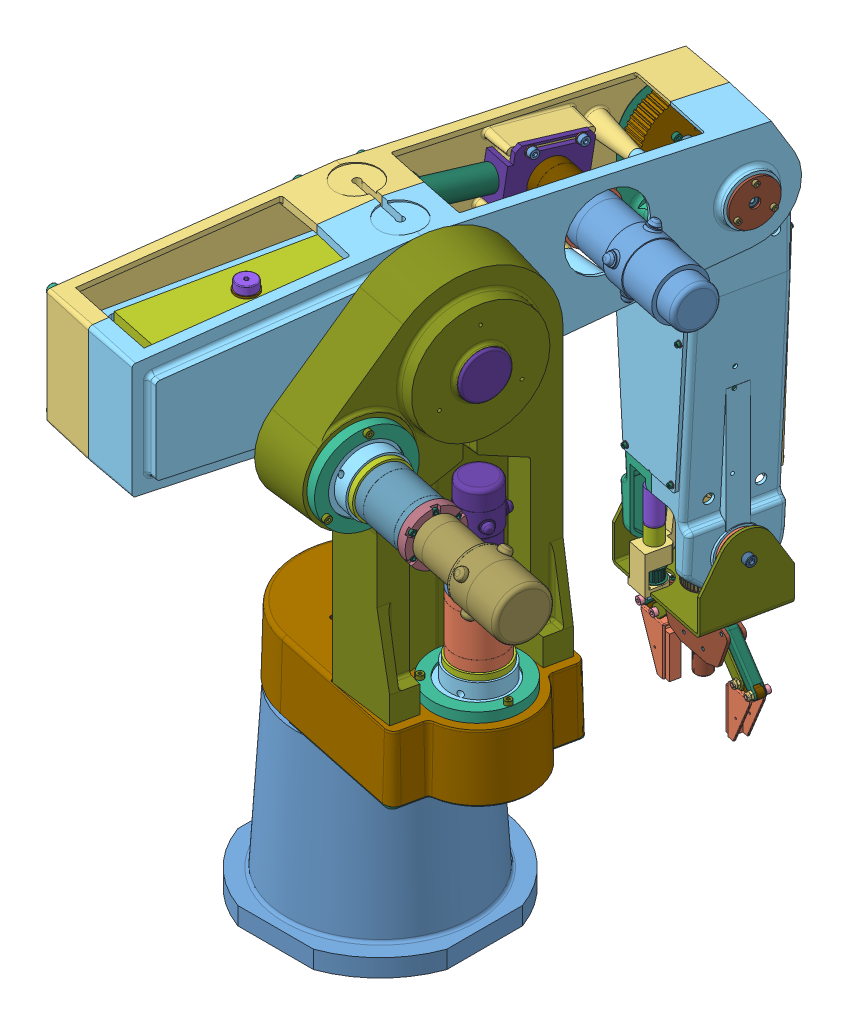
SolidWorks assembly Robot 2, configuration Défaut. Lengths in mm. (continued)
Components (placement in the parent): (continued)
- SE-AvtBras-1: SE-AvtBras [Défaut] at (55.1759 532.5 -274.5106) x (0 1 0) z (-0.978958 0 -0.204064) size (419.1 115.2 105.3)
  - AvtBrasD-1: AvtBrasD [Défaut] at origin size (406.26 90.38 52)
  - AvtBrasG-1: AvtBrasG [Défaut] at (-0.1665 0.8325 0) size (406.15 90.36 52)
  - parallel pin hardened_iso-1: parallel pin hardened_iso [Goupille  - 4 x 16 - A - St] at (-265.5 30.1675 -8) x (0 0 1) z (-0.010471 -0.999945 0) size (16 4 4)
  - Vis C HC, M 6x70-1: Vis C HC, M 6x70 [Défaut] at (-65 -16 45.5) x (1 0 0) z (0 -1 0) size (10 76 10)
  - GoupillePosition-1: GoupillePosition [Défaut] at (-65 -16 0.2) x (0 0 1) z (-0.991523 0.129934 0) size (10 8 8)
  - Support moteur-1: Support moteur [Défaut] at (-98.931 38.4675 -40.5) x (0 0 1) z (1 0 0) size (77 78 106) (hidden)
  - socket head cap screw_iso-1: socket head cap screw_iso [Vis CHC M5 x 12 --- 12N] at (-173.5 -4.3325 -27.8) x (0 0 -1) z (0.120643 0.992696 0) size (17 8.5 8.5)
  - socket head cap screw_iso-2: socket head cap screw_iso [Vis CHC M5 x 12 --- 12N] at (-153.5 -4.3325 -27.8) x (0 0 -1) z (0.975756 0.218862 0) size (17 8.5 8.5)
  - plain washer large grade ac_iso-1: plain washer large grade ac_iso [Rondelle M5 Washer ISO 7093 - 5] at (-173.5 -4.3325 -32.8) x (0 0 1) z (-1 0 0) size (1.2 15 15)
  - plain washer large grade ac_iso-3: plain washer large grade ac_iso [Rondelle M5 Washer ISO 7093 - 5] at (-153.5 -4.3325 -32.8) x (0 0 1) z (-1 0 0) size (1.2 15 15)
  - Poulie_M300-006-1: Poulie_M300-006 [Défaut] at (0 0 39) x (0 0 1) z (-0.707107 -0.707107 0) size (22 81.46 81.46)
  - Goupille Cylindrique type A  , 4x24-1: Goupille Cylindrique type A  , 4x24 [Défaut] at (9.1924 9.1924 26.3203) x (0.697271 -0.716808 0) z (0 0 1) size (4 4 24)
  - Goupille Cylindrique type A  , 4x24-3: Goupille Cylindrique type A  , 4x24 [Défaut] at (-9.1924 -9.1924 24.7225) x (-0.993131 -0.117006 0) z (0 0 1) size (4 4 24)
  - socket head cap screw_iso-3: socket head cap screw_iso [Vis CHC M4 x 25 ] at (-9.1924 9.1924 20) x (0 0 1) z (-1 0 0) size (29 7 7)
  - socket head cap screw_iso-4: socket head cap screw_iso [Vis CHC M4 x 25 ] at (9.1924 -9.1924 20) x (0 0 1) z (-1 0 0) size (29 7 7)
  - Came M300 008-1: Came M300 008 [Default] at (0 0 -43) x (0.999885 0.015178 0) z (0 0 1) size (76.42 80 10)
  - parallel pin hardened_iso-2: parallel pin hardened_iso [Goupille  - 4 x 16 - A - St] at (-6.5 -11.2583 -51.3276) x (0 0 1) z (-0.969957 0.243275 0) size (16 4 4)
  - socket head cap screw_iso-5: socket head cap screw_iso [CHC M4 x 16 --- 16N] at (-12.9985 -0.1973 -29) x (0 0 -1) z (-0.999639 0.026878 0) size (20 7 7)
  - socket head cap screw_iso-10: socket head cap screw_iso [CHC M4 x 16 --- 16N] at (6.6701 -11.1584 -29) x (0 0 -1) z (-0.999639 0.026878 0) size (20 7 7)
  - socket head cap screw_iso-12: socket head cap screw_iso [CHC M4 x 16 --- 16N] at (6.3284 11.3557 -29) x (0 0 -1) z (-0.999639 0.026878 0) size (20 7 7)
  - plain washer small grade a_iso-1: plain washer small grade a_iso [Washer M 4] at (-265.5 -21.8325 -8) x (0 0 1) z (-1 0 0) size (0.5 8 8)
  - socket head cap screw_iso-18: socket head cap screw_iso [CHC M4 x 16 --- 16N] at (-265.5 -21.8325 -12.5) x (0 0 1) z (-1 0 0) size (20 7 7)
  - plain washer small grade a_iso-3: plain washer small grade a_iso [Washer M 4] at (-265.5 23.1675 -8) x (0 0 1) z (-1 0 0) size (0.5 8 8)
  - socket head cap screw_iso-19: socket head cap screw_iso [CHC M4 x 16 --- 16N] at (-265.5 23.1675 -12.5) x (0 0 1) z (-1 0 0) size (20 7 7)
  - plain washer small grade a_iso-5: plain washer small grade a_iso [Washer M 4] at (-43.253 27.1675 -8) x (0 0 1) z (-1 0 0) size (0.5 8 8)
  - socket head cap screw_iso-20: socket head cap screw_iso [CHC M4 x 16 --- 16N] at (-43.253 27.1675 -12.5) x (0 0 1) z (-1 0 0) size (20 7 7)
  - moteur poignet-1: moteur poignet [Défaut] at (-218.4709 19.4675 19.5) size (70.8 35 35)
  - socket head cap screw_iso-21: socket head cap screw_iso [ISO 4762 M2 x 6 --- 6N] at (-174.931 8.4675 19.5) x (-1 0 0) z (0 0.924225 0.381849) size (8 3.8 3.8)
  - socket head cap screw_iso-22: socket head cap screw_iso [ISO 4762 M2 x 6 --- 6N] at (-174.931 19.4675 8.5) x (-1 0 0) z (0 -0.381849 0.924225) size (8 3.8 3.8)
  - socket head cap screw_iso-23: socket head cap screw_iso [ISO 4762 M2 x 6 --- 6N] at (-174.931 30.4675 19.5) x (-1 0 0) z (0 -0.924225 -0.381849) size (8 3.8 3.8)
  - socket head cap screw_iso-24: socket head cap screw_iso [ISO 4762 M2 x 6 --- 6N] at (-174.931 19.4675 30.5) x (-1 0 0) z (0 0.381849 -0.924225) size (8 3.8 3.8)
  - Vis CS, M 4x55-1: Vis CS, M 4x55 [Défaut] at (-88.5 -0.5325 -38.5) x (0 -1 0) z (0 0 1) size (7 57.41 7)
  - hex thin nut gradeb_iso-1: hex thin nut gradeb_iso [Hexagon Nut ISO - 4036 - M4 - N] at (-96.731 -0.5325 -38.5) x (0 -0.306361 -0.951915) z (1 0 0) size (7 8.08 2.2)
  - Accouplement flexible-1: Accouplement flexible [Default] at (-161.451 19.4675 19.5) x (-1 0 0) z (0 0.117803 -0.993037) size (17.76 9.53 9.53)
  - Codeur poignet-1: Codeur poignet [Défaut] at (-230.631 -7.9406 32.9669) x (0 0.056728 -0.99839) z (1 0 0) size (30 41.1 18.3)
  - RÇducteur-1: RÇducteur [Défaut] at (-143.931 29.4675 5.5) x (1 0 0) z (0 0 -1) size (82 70 28)
  - radial ball bearing_68_iso-1: radial ball bearing_68_iso [RBB - 1810 - 14,SI,NC,14_68] at (-317.5 -0.8325 -38.5) x (0 0 1) z (-0.812829 -0.582503 0) size (5 19 19)
  - plain washer small grade a_iso-6: plain washer small grade a_iso [Washer courte m5 7092 - 5] at (-138.931 7.4675 33.5) x (0 0 -1) z (1 0 0) size (1 9 9)
  - socket head cap screw_iso-25: socket head cap screw_iso [vis chc M5 x 35 --- 22N] at (-138.931 7.4675 39.5) x (0 0 -1) z (0.75446 0.656346 0) size (40 8.5 8.5)
  - plain washer small grade a_iso-7: plain washer small grade a_iso [Washer courte m5 7092 - 5] at (-88.931 7.4675 33.5) x (0 0 -1) z (1 0 0) size (1 9 9)
  - plain washer small grade a_iso-8: plain washer small grade a_iso [Washer courte m5 7092 - 5] at (-88.931 -35.5325 33.5) x (0 0 -1) z (1 0 0) size (1 9 9)
  - socket head cap screw_iso-26: socket head cap screw_iso [vis chc M5 x 35 --- 22N] at (-88.931 7.4675 39.5) x (0 0 -1) z (0.75446 0.656346 0) size (40 8.5 8.5)
  - socket head cap screw_iso-27: socket head cap screw_iso [vis chc M5 x 35 --- 22N] at (-88.931 -35.5325 39.5) x (0 0 -1) z (0.75446 0.656346 0) size (40 8.5 8.5)
  - Couvercle-3: Couvercle [Défaut] at (-317.5 -0.8325 -49.8) x (-0.559761 -0.828654 0) z (-0.828654 0.559761 0) size (41 8.8 41)
  - socket head cap screw_iso-28: socket head cap screw_iso [Vis CHC M3x8] at (-310.5 11.2918 -52.8) x (0 0 1) z (-0.923728 -0.383049 0) size (11 5.5 5.5)
  - socket head cap screw_iso-29: socket head cap screw_iso [Vis CHC M3x8] at (-310.5 -12.9569 -52.8) x (0 0 1) z (0.130134 0.991496 0) size (11 5.5 5.5)
  - socket head cap screw_iso-30: socket head cap screw_iso [Vis CHC M3x8] at (-331.5 -0.8325 -52.8) x (0 0 1) z (0.793594 -0.608447 0) size (11 5.5 5.5)
  - radial ball bearing_68_iso-4: radial ball bearing_68_iso [RBB - 1810 - 14,SI,NC,14_68] at (-317.5 -0.8325 38.2) x (0 0 1) z (-0.978908 -0.204302 0) size (5 19 19)
  - Couvercle-4: Couvercle [Défaut] at (-317.5 -0.8325 49.5) x (0.997516 0.070441 0) z (-0.070441 0.997516 0) size (41 8.8 41)
  - socket head cap screw_iso-31: socket head cap screw_iso [Vis CHC M3x8] at (-310.5 11.2918 52.5) x (0 0 -1) z (1 0 0) size (11 5.5 5.5)
  - socket head cap screw_iso-32: socket head cap screw_iso [Vis CHC M3x8] at (-331.5 -0.8325 52.5) x (0 0 -1) z (-0.5 0.866025 0) size (11 5.5 5.5)
  - socket head cap screw_iso-33: socket head cap screw_iso [Vis CHC M3x8] at (-310.5 -12.9569 52.5) x (0 0 -1) z (-0.5 -0.866025 0) size (11 5.5 5.5)
  - Capot Superieur_plexi-1: Capot Superieur_plexi [Défaut] at (-81.8928 43.8087 0) x (1 0 0) z (0 1 0) size (220 89.9 3.57)
  - plain washer 10673 type snl_iso-1: plain washer 10673 type snl_iso [rondelle M2] at (-264 46.4087 28) x (0 -1 0) z (0 0 1) size (0.6 6 6)
  - socket head cap screw_iso-34: socket head cap screw_iso [ISO 4762 M2.5 x 10 --- 10N] at (-264 48.9087 28) x (0 -1 0) z (0 0 1) size (12.5 4.5 4.5)
  - plain washer 10673 type snl_iso-9: plain washer 10673 type snl_iso [rondelle M2] at (-264 46.4087 -28) x (0 -1 0) z (0 0 1) size (0.6 6 6)
  - plain washer 10673 type snl_iso-11: plain washer 10673 type snl_iso [rondelle M2] at (-54 46.4087 -40) x (0 -1 0) z (0 0 1) size (0.6 6 6)
  - plain washer 10673 type snl_iso-13: plain washer 10673 type snl_iso [rondelle M2] at (-54 46.4087 40) x (0 -1 0) z (0 0 1) size (0.6 6 6)
  - socket head cap screw_iso-35: socket head cap screw_iso [ISO 4762 M2.5 x 10 --- 10N] at (-264 48.9087 -28) x (0 -1 0) z (0 0 1) size (12.5 4.5 4.5)
  - socket head cap screw_iso-36: socket head cap screw_iso [ISO 4762 M2.5 x 10 --- 10N] at (-54 48.9087 -40) x (0 -1 0) z (0 0 1) size (12.5 4.5 4.5)
  - socket head cap screw_iso-37: socket head cap screw_iso [ISO 4762 M2.5 x 10 --- 10N] at (-54 48.9087 40) x (0 -1 0) z (0 0 1) size (12.5 4.5 4.5)
  - Capot inferieur_plexi-1: Capot inferieur_plexi [Défaut] at (-207.8847 -47.4738 0) x (1 0 0) z (0 1 0) size (165 92.79 3.62)
  - plain washer 10673 type snl_iso-14: plain washer 10673 type snl_iso [rondelle M2] at (-121.3236 -48.0738 -40) x (0 1 0) z (-1 0 0) size (0.6 6 6)
  - plain washer 10673 type snl_iso-16: plain washer 10673 type snl_iso [rondelle M2] at (-121.3236 -48.0738 40) x (0 1 0) z (-1 0 0) size (0.6 6 6)
  - plain washer 10673 type snl_iso-18: plain washer 10673 type snl_iso [rondelle M2] at (-251.3236 -48.0738 30) x (0 1 0) z (-1 0 0) size (0.6 6 6)
  - plain washer 10673 type snl_iso-20: plain washer 10673 type snl_iso [rondelle M2] at (-251.3236 -48.0738 -30) x (0 1 0) z (-1 0 0) size (0.6 6 6)
  - socket head cap screw_iso-38: socket head cap screw_iso [ISO 4762 M2.5 x 10 --- 10N] at (-251.3236 -50.5738 -30) x (0 1 0) z (0 0 1) size (12.5 4.5 4.5)
  - socket head cap screw_iso-39: socket head cap screw_iso [ISO 4762 M2.5 x 10 --- 10N] at (-251.3236 -50.5738 30) x (0 1 0) z (0 0 -1) size (12.5 4.5 4.5)
  - socket head cap screw_iso-40: socket head cap screw_iso [ISO 4762 M2.5 x 10 --- 10N] at (-121.3236 -50.5738 40) x (0 1 0) z (0 0 -1) size (12.5 4.5 4.5)
  - socket head cap screw_iso-41: socket head cap screw_iso [ISO 4762 M2.5 x 10 --- 10N] at (-121.3236 -50.5738 -40) x (0 1 0) z (0 0 -1) size (12.5 4.5 4.5)
  - radial ball bearing_68_skf-1: radial ball bearing_68_skf [Roulement à billes 618-8] at (-113.931 -10.5325 -32.5) x (0 0 -1) z (1 0 0) size (4 16 16)
  - Arbre rÇducteur-1: Arbre rÇducteur [Défaut] at (-113.931 -10.5325 33.5) size (8 8 68)
  - Entretoise-1: Entretoise [Défaut] at (-113.931 -10.5325 -10.5) size (12 12 16)
- Arbre moteur Lacet-1: Arbre moteur Lacet [Défaut] at (123.3853 255.5 23.0723) x (0 -1 0) z (-0.495579 0 0.868563) size (78.5 36.84 36.92)
  - entraineur-1: entraineur [Défaut] at origin size (78.5 20 20)
  - PoulieE lacet-1: PoulieE lacet [Défaut] at (49 0 0) x (0 -1 0) z (-1 0 0) size (36.84 36.92 30)
  - socket set screw flat point_iso-1: socket set screw flat point_iso [ISO 4026 - M8 x 10-N] at (49 0 16.5) x (0 0 -1) z (1 0 0) size (10 8 8)
  - socket set screw flat point_iso-2: socket set screw flat point_iso [ISO 4026 - M8 x 10-N] at (-7.2554 0 12.9535) x (0 0 -1) z (0.96252 -0.271209 0) size (10 8 8)
- A-M_Epaule-1: A-M_Epaule [Défaut] at (103.905 474.5 118.9759) x (-0.978958 0 -0.204064) z (0.204064 0 -0.978958) size (78.5 36.84 36.92)
  - entraineur-1: entraineur [Défaut] at origin size (78.5 20 20)
  - P-E_Epaule-1: P-E_Epaule [Défaut] at (49 0 0) x (0 -1 0) z (-1 0 0) size (36.84 36.92 30)
  - socket set screw flat point_iso-1: socket set screw flat point_iso [ISO 4026 - M8 x 10-N] at (49 0 16.5) x (0 0 -1) z (1 0 0) size (10 8 8)
  - socket set screw flat point_iso-2: socket set screw flat point_iso [ISO 4026 - M8 x 10-N] at (-7.2554 0 12.9535) x (0 0 -1) z (0.96252 -0.271209 0) size (10 8 8)
- Poulie_M300-007-1: Poulie_M300-007 [Défaut] at (11.0359 549.2909 -160.7657) x (0.978958 0 0.204064) z (-0.164446 -0.592111 0.7889) size (27 22.5 22.65)
- Poulie Poignet-1: Poulie Poignet [Défaut] at (73.0952 418.569 -260.0164) x (0.204064 0 -0.978958) z (0.978958 0 0.204064) size (27.43 27.43 20)
- poulie pivotement poignet-1: poulie pivotement poignet [Défaut] at (28.274 174.3879 -250.512) x (-0.99945 0 0.033175) z (0 -1 0) size (20 20 14)
- Support_poignet-1: Support_poignet [Défaut] at (55.006 215 -273.6956) x (0 1 0) z (-0.978958 0 -0.204064) size (98.66 84.05 127)
  - Support-1: Support [Défaut] at origin size (81.5 81.2 115)
  - Assemblage axe pince-1: Assemblage axe pince [Défaut] at (-13.5 0 0) x (0 0 -1) z (1 0 0) size (109 40 59)
    - partie centrale axe avant bras-1: partie centrale axe avant bras [Défaut] at origin size (12 40 21)
    - intÇrieur piäce centrale-1: intÇrieur piäce centrale [Défaut] at (-3 1.5 5) size (6 15.94 13)
    - intÇrieur piäce centrale-2: intÇrieur piäce centrale [Défaut] at (3 -1.5 5) x (-1 0 0) z (0 0 1) size (6 15.94 13)
    - cotÇ axe avant bras-1: cotÇ axe avant bras [Défaut] at (-6 1.807 8.3053) x (1 0 0) z (0 0.944488 0.328546) size (48.5 11 11)
    - cotÇ axe avant bras-2: cotÇ axe avant bras [Défaut] at (6 -1.6292 8.2468) x (-1 0 0) z (0 -0.95512 0.296219) size (48.5 11 11)
    - axe roulements-1: axe roulements [Défaut] x (0 0 -1) z (0.989499 0.144542 0) size (38 10.89 10.89)
  - Assemblage support moteur-1: Assemblage support moteur [Défaut] at (-44.3507 -38.7833 30.5386) x (-1 0 0) z (0 0 -1) size (78.32 60.15 22.52)
    - Support moteur + axe-1: Support moteur + axe [Défaut] at origin size (75.82 60.15 22.2)
    - capteur sur support moteur-1: capteur sur support moteur [Défaut] at (-40.0112 47.5459 15.95) x (0 -0.781659 -0.623706) z (1 0 0) size (6.5 6.5 27.6)
    - plaque avant support moteur-1: plaque avant support moteur [Défaut] at (14.8869 1.1807 -1.9) x (0 0 -1) z (1 0 0) size (22 24 2.5)
  - Ecrou hexagonal ISO 4032, M 9-1: Ecrou hexagonal ISO 4032, M 9 [Défaut] at (-44.23 0 0) x (0 1 0) z (0 0 1) size (16.17 6.98 14)
  - moteur pivotement poignet-1: moteur pivotement poignet [Défaut] at (-26.4843 -28.1507 21.4386) x (-1 0 0) z (0 -0.157023 -0.987595) size (81.2 19.59 19.59)
    - rÇducteur micromoteur-1: rÇducteur micromoteur [Défaut] at origin size (48.3 16 16)
    - micromoteur-1: micromoteur [Défaut] at (-2.1408 0 0) x (1 0 0) z (0 -0.965969 0.258658) size (41 16 16)
  - Poulie axe poignet-1: Poulie axe poignet [Défaut] at (0 0 -18.0612) x (-0.954858 -0.297063 0) z (0 0 -1) size (58.99 58.99 20)
  - Vis C HC, M 6x16-1: Vis C HC, M 6x16 [Défaut] at (0 0 57.5) x (0.243653 -0.969862 0) z (-0.969862 -0.243653 0) size (10 22.04 10)
  - Vis C HC, M 6x16-2: Vis C HC, M 6x16 [Défaut] at (0 0 -57.5) x (1 0 0) z (0 1 0) size (10 22.04 10)
- PortePince-1: PortePince [Défaut] at (55.006 215 -273.6956) x (0 1 0) z (-0.204064 0 0.978958) size (147.79 157.25 45.47)
  - Corps_poignet-1: Corps_poignet [Défaut] at (-113.4 0 -8.5) x (0 -1 0) z (0 0 1) size (87.98 118.07 45.47)
    - Main-1: Main [Défaut] at origin size (87.98 81.17 33)
    - fourreau de poignet-1: fourreau de poignet [Défaut] at (0 76.4 8.5) x (0 1 0) z (0.435216 0 0.900326) size (46.9 34.05 34.05)
    - Roulement type BC 9x17x4-1: Roulement type BC 9x17x4 [Défaut] at (0 94.9 8.5) x (0 -1 0) z (-0.453716 0 0.891146) size (4 17 17)
    - Roulement type BC 9x17x4-2: Roulement type BC 9x17x4 [Défaut] at (0 71.1711 8.5) x (0 -1 0) z (0 0 1) size (4 17 17)
    - Axe-goupille-1: Axe-goupille [Défaut] at (36.5 37 17) size (3.5 3.5 17)
    - Axe-goupille-2: Axe-goupille [Défaut] at (18.5 37 17) size (3.5 3.5 17)
    - Axe-goupille-3: Axe-goupille [Défaut] at (-18.5 37 17) size (3.5 3.5 17)
    - Axe-goupille-4: Axe-goupille [Défaut] at (-36.5 37 17) size (3.5 3.5 17)
    - Axe-goupille-5: Axe-goupille [Défaut] at (-12.5 10 17) size (3.5 3.5 17)
    - Axe-goupille-6: Axe-goupille [Défaut] at (12.5 10 17) size (3.5 3.5 17)
  - bielle 1-1: bielle 1 [Défaut] at (-106.9547 -75.1317 5.4) x (-0.717304 0.69676 0) z (0 0 -1) size (9.87 58.75 10.8)
  - bielle 1-2: bielle 1 [Défaut] at (-106.9547 75.1317 -5.4) x (-0.717304 -0.69676 0) z (0 0 1) size (9.87 58.75 10.8)
  - bielle 2-1: bielle 2 [Défaut] at (-80.8832 -14.1453 5.4) x (0.717304 -0.69676 0) z (0 0 -1) size (12.5 61.5 10.8)
    - bielle 2-1: bielle 2 [Défaut] at origin size (12.5 61.5 10.8)
    - goupille bielle 2-1: goupille bielle 2 [Défaut] at (6.25 18 10.8) x (-0.698934 -0.715186 0) z (0 0 1) size (3.5 3.5 10.8)
  - bielle 2-2: bielle 2 [Défaut] at (-80.8832 14.1453 -5.4) x (0.717304 0.69676 0) z (0 0 1) size (12.5 61.5 10.8)
    - bielle 2-1: bielle 2 [Défaut] at origin size (12.5 61.5 10.8)
    - goupille bielle 2-1: goupille bielle 2 [Défaut] at (6.25 18 10.8) x (-0.698934 -0.715186 0) z (0 0 1) size (3.5 3.5 10.8)
  - Mors-3: Mors [Défaut] at (-210.2541 103.6501 -0.5) x (-1 0 0) z (0 0 -1) size (60 39.8 20)
    - Bielle 3-1: Bielle 3 [Défaut] at (-104.4629 -50.0022 -4.6) size (9.5 27.5 8.2)
    - goupille-1: goupille [Défaut] at (-106.9629 -37.5022 -0.5) x (0 -0.527582 0.849504) z (-1 0 0) size (4 4 14)
    - mors-1: mors [Défaut] at (-49.5801 -64.5882 6.5) size (48 34 14)
    - ecrou_uni_7474-m4x0_7-4_8-5s-1: ecrou_uni_7474-m4x0_7-4_8-5s [Défaut] at (-99.7129 -32.0022 4.9) x (0.66757 0.744547 0) z (0 0 1) size (7 8.09 4.8)
    - ecrou_uni_7474-m4x0_7-4_8-5s-2: ecrou_uni_7474-m4x0_7-4_8-5s [Défaut] at (-99.7129 -50.0022 4.9) x (0.967807 0.251692 0) z (0 0 1) size (7 8.09 4.8)
    - vis chc M4x16-1: vis chc M4x16 [Default] at (-99.7129 -32.0022 -5.9) x (0.255972 0.966684 0) z (0 0 1) size (7 7 20)
    - vis chc M4x16-2: vis chc M4x16 [Default] at (-99.7129 -50.0022 -5.9) x (-0.658187 0.752854 0) z (0 0 1) size (7 7 20)
    - Vis Chc M4-1: Vis Chc M4 [Default] at (-92.9629 -44.5022 -0.5) x (0 0 1) z (-1 0 0) size (7 7 16)
  - Mors-4: Mors [Défaut] at (-210.2541 -103.6501 0.5) x (-1 0 0) z (0 0 1) size (60 39.8 20)
    - Bielle 3-1: Bielle 3 [Défaut] at (-104.4629 -50.0022 -4.6) size (9.5 27.5 8.2)
    - goupille-1: goupille [Défaut] at (-106.9629 -37.5022 -0.5) x (0 -0.527582 0.849504) z (-1 0 0) size (4 4 14)
    - mors-1: mors [Défaut] at (-49.5801 -64.5882 6.5) size (48 34 14)
    - ecrou_uni_7474-m4x0_7-4_8-5s-1: ecrou_uni_7474-m4x0_7-4_8-5s [Défaut] at (-99.7129 -32.0022 4.9) x (0.66757 0.744547 0) z (0 0 1) size (7 8.09 4.8)
    - ecrou_uni_7474-m4x0_7-4_8-5s-2: ecrou_uni_7474-m4x0_7-4_8-5s [Défaut] at (-99.7129 -50.0022 4.9) x (0.967807 0.251692 0) z (0 0 1) size (7 8.09 4.8)
    - vis chc M4x16-1: vis chc M4x16 [Default] at (-99.7129 -32.0022 -5.9) x (0.255972 0.966684 0) z (0 0 1) size (7 7 20)
    - vis chc M4x16-2: vis chc M4x16 [Default] at (-99.7129 -50.0022 -5.9) x (-0.658187 0.752854 0) z (0 0 1) size (7 7 20)
    - Vis Chc M4-1: Vis Chc M4 [Default] at (-92.9629 -44.5022 -0.5) x (0 0 1) z (-1 0 0) size (7 7 16)
Mates (geometry in assembly coordinates):
- Coaxiale1: concentric aligned: cylinder of Ens_Socle-1/Fourreau_200-604-1 through (0 221.7474 0) axis (0 1 0) radius 23.5; cylinder of SE_Chaise-1/SE-Assise-1/SKF_7204-2 through (0 165.3625 0) axis (0 1 0) radius 23.5
- Coïncidente1: coincident anti-aligned: plane of Ens_Socle-1/Fourreau_200-604-1 through (-1.9708 229.5 23.4172) normal (0 -1 0); plane of SE_Chaise-1/SE-Assise-1/SKF_7204-1 through (20.3378 229.5 4.2394) normal (0 1 0)
- Coaxiale2: concentric anti-aligned: cylinder of SE_Chaise-1/Dossier-1 through (63.6282 532.5 13.2698) axis (0.978958 0 0.204064) radius 23.5; cylinder of Bras-1/AXE_Bras-1/7204_Rlt-Billes-2 through (138.1636 532.5 28.8067) axis (-0.978958 0 -0.204064) radius 23.5
- Coïncidente2: coincident anti-aligned: plane of SE_Chaise-1/Dossier-1 through (124.8131 532.5 26.0238) normal (-0.978958 0 -0.204064); plane of Bras-1/AXE_Bras-1/7204_Rlt-Billes-2 through (122.0035 548.0575 39.5023) normal (0.978958 0 0.204064)
- Coaxiale3: concentric aligned: cylinder of Bras-1/AXE 04 021 M300 011-1 through (-5.5195 532.5 -287.1625) axis (0.978958 0 0.204064) radius 6; cylinder of SE-AvtBras-1/AvtBrasG-1 through (4.2701 532.5 -285.1219) axis (0.978958 0 0.204064) radius 6
- Coïncidente3: coincident aligned: plane of Bras-1/BrasDroit-2 through (-3.3238 505.7717 6.1308) normal (-0.978958 0 -0.204064); plane of SE-AvtBras-1/AvtBrasD-1 through (55.1759 532.5 -274.5106) normal (-0.978958 0 -0.204064)
- Coaxiale5: concentric aligned: cylinder of SE_Chaise-1/Moto-rÇducteur lacet-1/SKF 6002-1 through (123.3853 209.2625 23.0723) axis (0 1 0) radius 7.5; cylinder of Arbre moteur Lacet-1/entraineur-1 through (123.3853 277.7027 23.0723) axis (0 1 0) radius 7.5
- Coïncidente5: coincident anti-aligned: plane of SE_Chaise-1/Moto-rÇducteur lacet-1/SKF 6002-2 through (125.8248 255.5 30.481) normal (0 1 0); plane of Arbre moteur Lacet-1/entraineur-1 through (132.071 255.5 28.028) normal (0 -1 0)
- Coaxiale6: concentric aligned: cylinder of SE_Chaise-1/Moteur Epaule-1/SKF 6002-2 through (58.6404 474.5 109.5405) axis (0.978958 0 0.204064) radius 7.5; cylinder of A-M_Epaule-1/entraineur-1 through (125.6404 474.5 123.5067) axis (0.978958 0 0.204064) radius 7.5
- Coïncidente6: coincident anti-aligned: plane of SE_Chaise-1/Moteur Epaule-1/SKF 6002-1 through (102.3345 473.2287 126.5097) normal (0.978958 0 0.204064); plane of A-M_Epaule-1/entraineur-1 through (103.905 484.5 118.9759) normal (-0.978958 0 -0.204064)
- Coaxiale7: concentric anti-aligned: cylinder of Bras-1/MotoReduc_Coude-1/Sortie reduc-1 through (11.5254 549.2909 -160.6637) axis (0.978958 0 0.204064) radius 5; cylinder of Poulie_M300-007-1 through (-0.961 549.2909 -163.2665) axis (-0.978958 0 -0.204064) radius 5
- Coaxiale8: concentric aligned: cylinder of Bras-1/MotoReduc_Coude-1/Sortie reduc-1 through (-3.8052 552.2514 -167.9753) axis (-0.164446 -0.592111 0.7889) radius 1.5; cylinder of Poulie_M300-007-1 through (-2.7651 555.9965 -172.965) axis (-0.164446 -0.592111 0.7889) radius 1.5
- Coaxiale9: concentric aligned: cylinder of SE-AvtBras-1/Arbre rÇducteur-1 through (86.8006 418.569 -257.1595) axis (-0.978958 0 -0.204064) radius 4; cylinder of Poulie Poignet-1 through (82.8848 418.569 -257.9757) axis (-0.978958 0 -0.204064) radius 4
- Coïncidente7: coincident anti-aligned: plane of SE-AvtBras-1/Entretoise-1 through (63.3057 418.569 -262.057) normal (0.978958 0 0.204064); plane of Poulie Poignet-1 through (63.3057 418.569 -262.057) normal (-0.978958 0 -0.204064)
- Coaxiale10: concentric anti-aligned: cylinder of Support_poignet-1/Assemblage axe pince-1/axe roulements-1 through (55.006 163.5 -273.6956) axis (0 1 0) radius 4.5; cylinder of PortePince-1/Corps_poignet-1/fourreau de poignet-1 through (55.006 146.4624 -273.6956) axis (0 -1 0) radius 11
- Coaxiale11: concentric anti-aligned: cylinder of Support_poignet-1/Assemblage axe pince-1/cotÇ axe avant bras-2 through (90.2485 215 -266.3493) axis (0.978958 0 0.204064) radius 5; cylinder of SE-AvtBras-1/radial ball bearing_68_iso-1 through (112.8991 215 -261.6278) axis (-0.978958 0 -0.204064) radius 5
- Coïncidente8: coincident aligned: plane of SE-AvtBras-1/AvtBrasD-1 through (55.1759 532.5 -274.5106) normal (-0.978958 0 -0.204064); plane of Support_poignet-1/Support-1 through (55.006 215 -273.6956) normal (-0.978958 0 -0.204064)
- Coïncidente9: coincident anti-aligned: plane of Support_poignet-1/Assemblage axe pince-1/axe roulements-1 through (55.006 198.5 -273.6956) normal (0 -1 0); plane of PortePince-1/Corps_poignet-1/Roulement type BC 9x17x4-1 through (58.8271 198.5 -270.6281) normal (0 1 0)
- Coaxiale12: concentric aligned: cylinder of poulie pivotement poignet-1 through (28.274 162.3879 -250.512) axis (0 1 0) radius 1.5; cylinder of Support_poignet-1/moteur pivotement poignet-1/rÇducteur micromoteur-1 through (28.274 253.1757 -250.512) axis (0 1 0) radius 1.5
- Coïncidente10: coincident anti-aligned: plane of poulie pivotement poignet-1 through (28.274 174.3879 -250.512) normal (0 1 0); plane of Support_poignet-1/moteur pivotement poignet-1/rÇducteur micromoteur-1 through (29.3794 174.3879 -253.4207) normal (0 -1 0)
- Parallèle3: parallel anti-aligned: plane of Ens_Socle-1/Socle-1 through (-113 0 0) normal (0 -1 0); plane of Bras-1/BrasDroit-2
- Parallèle2: parallel aligned: plane of SE-AvtBras-1/AvtBrasD-1; plane of Support_poignet-1/Support-1
- Perpendiculaire1: perpendicular: plane of Ens_Socle-1/Socle-1 through (-113 0 0) normal (0 -1 0); plane of SE-AvtBras-1/AvtBrasD-1
- Coïncidente16: coincident anti-aligned: plane of Support_poignet-1/Support-1; plane of PortePince-1 through (55.006 215 -273.6956) normal (-0.204064 0 0.978958)
